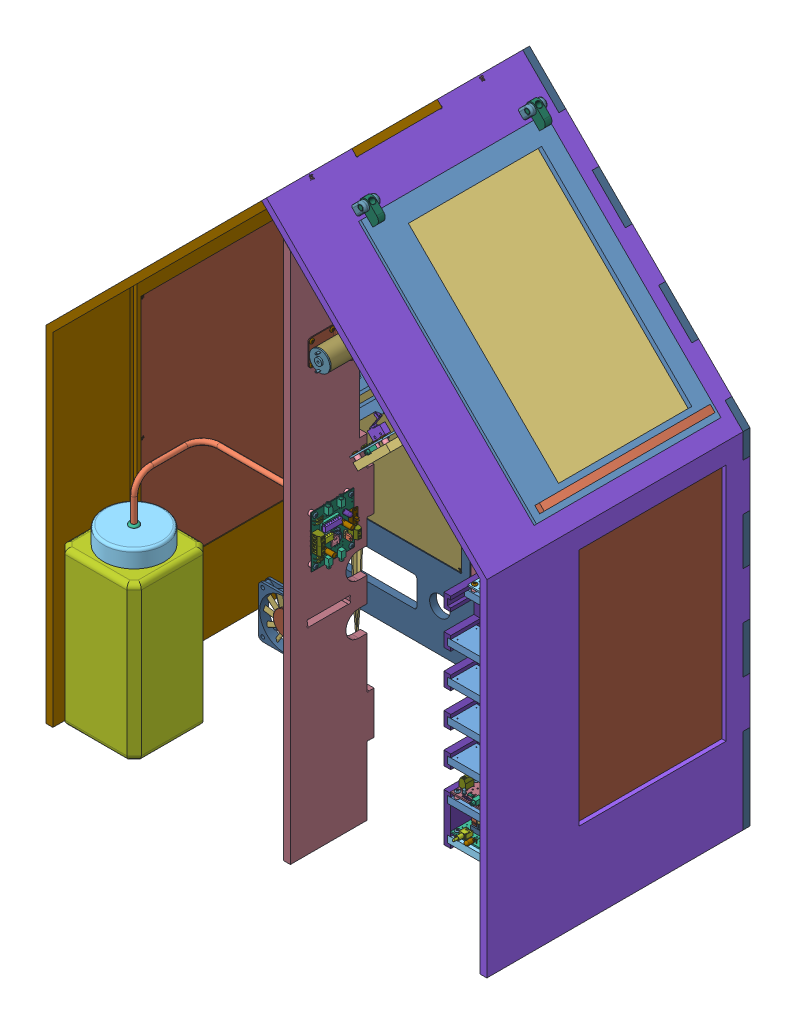
SolidWorks assembly Serre de base VDS, configuration guillotine. Lengths in mm. (continued)
Components (placement in the parent): (continued)
- Cache Oled-2: Cache Oled [Défaut] at (-241.7989 -284.4707 -216) (hidden)
- guillotine-1: guillotine [Défaut] at (-150.376 -16.7665 73.5) (hidden)
- Sonde capteur humidité-1: Sonde capteur humidité [Défaut] at (349.3697 -143.9656 -111.3159) x (1 0 0) z (0 1 0) size (30.38 36.99 53.6) (hidden)
  - Base capteur humidité terre-1: Base capteur humidité terre [Défaut] at (-210.4875 -4.2437 -4) size (29.6 36.6 12.37)
  - Capot capteur humidité terre-1: Capot capteur humidité terre [Défaut] at (-210.4875 -4.2437 32.3863) x (0 0 1) z (-0.999641 -0.026785 0) size (7 29.6 29.6)
  - Tige capteur humidité-1: Tige capteur humidité [Défaut] at (-221.4875 -4.2437 8) x (1 0 0) z (0 1 0) size (3 50 3)
  - Tige capteur humidité-2: Tige capteur humidité [Défaut] at (-199.4875 -4.2437 8) x (1 0 0) z (0 1 0) size (3 50 3)
  - CI capteur humidité terre-1: CI capteur humidité terre [Défaut] at (-210.4875 -4.2437 3) size (25.6 25.6 1.6)
  - Vis 2.2 x 9.5-1: Vis 2.2 x 9.5 [Défaut] at (-210.4875 -4.2437 9.6) x (0.624792 0.780791 0) z (0.780791 -0.624792 0) size (4.27 12.1 4.27)
  - Résistance 75 Kohm Pas de 10-1: Résistance 75 Kohm Pas de 10 [Défaut] at (-210.4875 -12.0088 0.7228) x (1 0 0) z (0 1 0) size (10.5 4.15 2.3)
Mates (geometry in assembly coordinates):
- Coïncidente1: coincident anti-aligned: axis of FONDINTERIEUR-1 through (57.939 191.6778 -4) axis (0 0 1); axis of Rondelle métal 3 x 12-1 through (57.939 191.6778 8.8) axis (0 0 -1)
- Coïncidente2: coincident anti-aligned: axis of Rondelle métal 3 x 12-1 through (57.939 191.6778 8.8) axis (0 0 -1); axis of VIs TC 3 x 13-1 through (57.939 191.6778 -1.7) axis (0 0 1)
- Coïncidente3: coincident anti-aligned: axis of FONDINTERIEUR-1 through (22.5836 156.3225 -4) axis (0 0 1); axis of Rondelle métal 3 x 12-2 through (22.5836 156.3225 8.8) axis (0 0 -1)
- Coïncidente4: coincident anti-aligned: axis of VIs TC 3 x 13-2 through (22.5836 156.3225 -1.7) axis (0 0 1); axis of Rondelle métal 3 x 12-2 through (22.5836 156.3225 8.8) axis (0 0 -1)
- Coïncidente5: coincident aligned: circle of VIs TC 3 x 13-2; plane of Rondelle métal 3 x 12-2 through (22.5836 156.3225 8.8) normal (0 0 1)
- Coïncidente6: coincident anti-aligned: plane of Rondelle métal 3 x 12-1 through (57.939 191.6778 8.8) normal (0 0 1); plane of VIs TC 3 x 13-1 through (57.939 191.6778 8.8) normal (0 0 -1)
- Coïncidente14: coincident anti-aligned: axis of FONDINTERIEUR-1 through (57.939 191.6778 -4) axis (0 0 1); axis of Entretoise CI-1 through (57.939 191.6778 8.1) axis (0 0 -1)
- Coïncidente15: coincident aligned: plane of FONDINTERIEUR-1 through (-297.9367 -225.0262 4) normal (0 0 1); circle of Entretoise CI-1
- Coïncidente16: coincident anti-aligned: axis of FONDINTERIEUR-1 through (22.5836 156.3225 -4) axis (0 0 1); axis of Entretoise CI-2 through (22.5836 156.3225 8.1) axis (0 0 -1)
- Coïncidente17: coincident aligned: plane of FONDINTERIEUR-1 through (-297.9367 -225.0262 4) normal (0 0 1); circle of Entretoise CI-2
- Tangent4: tangent anti-aligned: plane of Crémallière M3-3-1 through (-72.5742 65.3366 12) normal (0.707107 -0.707107 0); cylinder of Entretoise CI-2 through (22.5836 156.3225 8.1) axis (0 0 -1) radius 2.95
- Parallèle1: parallel aligned: plane of FONDINTERIEUR-1 through (-307.876 77.2771 4) normal (-0.707107 0.707107 0); plane of Crémallière M3-3-1 through (-52.7752 102.1062 12) normal (-0.707107 0.707107 0)
- Coïncidente19: coincident anti-aligned: plane of FONDINTERIEUR-1 through (-297.9367 -225.0262 4) normal (0 0 1); plane of Crémallière M3-3-1 through (65.6965 199.3646 4) normal (0 0 -1)
- Coïncidente20: coincident aligned: axis of FONDINTERIEUR-1 through (57.939 191.6778 -4) axis (0 0 1); axis of VIs TC 3 x 13-1 through (57.939 191.6778 -1.7) axis (0 0 1)
- Coïncidente21: coincident anti-aligned: plane of Crémallière M3-3-1 through (-70.4528 63.2153 8) normal (0 0 1); plane of Rondelle métal 3 x 12-1 through (57.939 191.6778 8) normal (0 0 -1)
- Coïncidente22: coincident anti-aligned: plane of Crémallière M3-3-1 through (-70.4528 63.2153 8) normal (0 0 1); plane of Rondelle métal 3 x 12-2 through (22.5836 156.3225 8) normal (0 0 -1)
- Coïncidente23: coincident anti-aligned: plane of FONDINTERIEUR-1 through (62.7794 136.4142 -4) normal (0.707107 -0.707107 0); plane of Prépa 06 module Microrupteur-1/support capteur-1 through (87.5711 161.2058 2.9393) normal (-0.707107 0.707107 0)
- Coïncidente24: coincident anti-aligned: plane of FONDINTERIEUR-1 through (96.8921 167.5269 -4) normal (-0.707107 -0.707107 0); plane of Prépa 06 module Microrupteur-1/support capteur-1 through (95.3921 169.0269 -4) normal (0.707107 0.707107 0)
- Coïncidente25: coincident aligned: plane of FONDINTERIEUR-1 through (-297.9367 -225.0262 -4) normal (0 0 -1); plane of Prépa 06 module Microrupteur-1/support capteur-1 through (95.3921 169.0269 -4) normal (0 0 -1)
- Coïncidente26: coincident anti-aligned: plane of FONDINTERIEUR-1 through (-7.9312 65.7035 -4) normal (0.707107 -0.707107 0); plane of Prépa 06 module Microrupteur-2/support capteur-1 through (16.8604 90.4952 2.9393) normal (-0.707107 0.707107 0)
- Coïncidente27: coincident anti-aligned: plane of FONDINTERIEUR-1 through (26.1815 96.8162 -4) normal (-0.707107 -0.707107 0); plane of Prépa 06 module Microrupteur-2/support capteur-1 through (24.6815 98.3162 -4) normal (0.707107 0.707107 0)
- Coïncidente28: coincident aligned: plane of FONDINTERIEUR-1 through (-297.9367 -225.0262 -4) normal (0 0 -1); plane of Prépa 06 module Microrupteur-2/support capteur-1 through (24.6815 98.3162 -4) normal (0 0 -1)
- Coïncidente29: coincident anti-aligned: axis of FONDINTERIEUR-1 through (-138.876 -138.9656 -4) axis (0 0 1); axis of Ventilateur-1/Cage ventilateur-1 through (-138.876 -138.9656 14.4) axis (0 0 -1)
- Coïncidente30: coincident anti-aligned: axis of FONDINTERIEUR-1 through (-88.876 -138.9656 -4) axis (0 0 1); axis of Ventilateur-1/Cage ventilateur-1 through (-88.876 -138.9656 14.4) axis (0 0 -1)
- Coïncidente31: coincident: plane of FONDINTERIEUR-1 through (-297.9367 -225.0262 4) normal (0 0 1); line of Ventilateur-1/Cage ventilateur-1 through (-143.876 -138.9656 4) axis (0 -1 0)
- Coïncidente32: coincident anti-aligned: axis of Ventilateur-1/Cage ventilateur-1 through (-138.876 -138.9656 14.4) axis (0 0 -1); axis of VIs TC 3 x 13-4 through (-138.876 -138.9656 3.9) axis (0 0 1)
- Coïncidente33: coincident anti-aligned: axis of Ventilateur-1/Cage ventilateur-1 through (-88.876 -138.9656 14.4) axis (0 0 -1); axis of VIs TC 3 x 13-6 through (-88.876 -138.9656 3.9) axis (0 0 1)
- Coïncidente34: coincident anti-aligned: axis of Ventilateur-1/Cage ventilateur-1 through (-88.876 -188.9656 14.4) axis (0 0 -1); axis of VIs TC 3 x 13-7 through (-88.876 -188.9656 3.9) axis (0 0 1)
- Coïncidente35: coincident anti-aligned: axis of Ventilateur-1/Cage ventilateur-1 through (-138.876 -188.9656 14.4) axis (0 0 -1); axis of VIs TC 3 x 13-8 through (-138.876 -188.9656 3.9) axis (0 0 1)
- Coïncidente36: coincident aligned: plane of Ventilateur-1/Cage ventilateur-1 through (-88.876 -138.9656 14.4) normal (0 0 1); circle of VIs TC 3 x 13-8
- Coïncidente37: coincident aligned: plane of Ventilateur-1/Cage ventilateur-1 through (-88.876 -138.9656 14.4) normal (0 0 1); circle of VIs TC 3 x 13-4
- Coïncidente38: coincident aligned: plane of Ventilateur-1/Cage ventilateur-1 through (-88.876 -138.9656 14.4) normal (0 0 1); circle of VIs TC 3 x 13-6
- Coïncidente39: coincident aligned: plane of Ventilateur-1/Cage ventilateur-1 through (-88.876 -138.9656 14.4) normal (0 0 1); circle of VIs TC 3 x 13-7
- Coïncidente40: coincident aligned: axis of FONDINTERIEUR-1 through (8.418 76.3959 4) axis (0 0 -1); axis of VIS TORCX TF 3 X 19-2 through (8.418 76.3959 12.4885) axis (0 0 -1)
- Coïncidente41: coincident aligned: plane of FONDINTERIEUR-1 through (-297.9367 -225.0262 -4) normal (0 0 -1); plane of VIS TORCX TF 3 X 19-2 through (7.3455 78.9824 -4) normal (0 0 -1)
- Coïncidente42: coincident aligned: axis of FONDINTERIEUR-1 through (79.1287 147.1066 4) axis (0 0 -1); axis of VIS TORCX TF 3 X 19-1 through (79.1287 147.1066 12.4885) axis (0 0 -1)
- Coïncidente43: coincident aligned: plane of FONDINTERIEUR-1 through (-297.9367 -225.0262 -4) normal (0 0 -1); plane of VIS TORCX TF 3 X 19-1 through (78.0561 149.693 -4) normal (0 0 -1)
- Coïncidente44: coincident anti-aligned: plane of FONDINTERIEUR-1 through (-26.876 223.1558 -4) normal (-1 0 0); plane of Prépa 02 renfort arrière-1/renfortarriere-1 through (-26.876 272.0951 2.9393) normal (1 0 0)
- Coïncidente45: coincident anti-aligned: plane of FONDINTERIEUR-1 through (-28.9973 271.0344 -4) normal (0 -1 0); plane of Prépa 02 renfort arrière-1/renfortarriere-1 through (-26.876 271.0344 -4) normal (0 1 0)
- Coïncidente46: coincident aligned: plane of FONDINTERIEUR-1 through (-297.9367 -225.0262 -4) normal (0 0 -1); plane of Prépa 02 renfort arrière-1/renfortarriere-1 through (-26.876 221.1086 -4) normal (0 0 -1)
- Coïncidente47: coincident anti-aligned: plane of FONDINTERIEUR-1 through (-56.9973 -85.9656 -4) normal (0 -1 0); plane of étagèrebrumi-1 through (-297.9367 -85.9656 72.872) normal (0 1 0)
- Coïncidente48: coincident anti-aligned: plane of FONDINTERIEUR-1 through (-54.876 -88.0869 -4) normal (-1 0 0); plane of étagèrebrumi-1 through (-54.876 -85.9656 1.8787) normal (1 0 0)
- Coïncidente49: coincident aligned: plane of FONDINTERIEUR-1 through (-297.9367 -225.0262 -4) normal (0 0 -1); plane of étagèrebrumi-1 through (-54.876 -85.9656 -4) normal (0 0 -1)
- Coïncidente50: coincident anti-aligned: axis of FONDINTERIEUR-1 through (-30.876 -315.9656 -4) axis (0 0 1); axis of VIS TORCX TF 3 X 19-3 through (-30.876 -315.9656 12.4885) axis (0 0 -1)
- Coïncidente51: coincident aligned: plane of FONDINTERIEUR-1 through (-297.9367 -225.0262 -4) normal (0 0 -1); plane of VIS TORCX TF 3 X 19-3 through (-31.2492 -313.1905 -4) normal (0 0 -1)
- Coïncidente52: coincident anti-aligned: axis of FONDINTERIEUR-1 through (-30.876 -274.5499 -4) axis (0 0 1); axis of VIS TORCX TF 3 X 19-4 through (-30.876 -274.5499 12.4885) axis (0 0 -1)
- Coïncidente53: coincident aligned: plane of FONDINTERIEUR-1 through (-297.9367 -225.0262 -4) normal (0 0 -1); plane of VIS TORCX TF 3 X 19-4 through (-31.2492 -271.7749 -4) normal (0 0 -1)
- Coïncidente54: coincident anti-aligned: axis of FONDINTERIEUR-1 through (-169.876 -89.9656 -4) axis (0 0 1); axis of VIS TORCX TF 3 X 19-5 through (-169.876 -89.9656 12.4885) axis (0 0 -1)
- Coïncidente55: coincident aligned: plane of FONDINTERIEUR-1 through (-297.9367 -225.0262 -4) normal (0 0 -1); plane of VIS TORCX TF 3 X 19-5 through (-170.2492 -87.1905 -4) normal (0 0 -1)
- Coïncidente56: coincident anti-aligned: axis of FONDINTERIEUR-1 through (-30.876 -27.0369 -4) axis (0 0 1); axis of VIS TORCX TF 3 X 19-6 through (-30.876 -27.0369 12.4885) axis (0 0 -1)
- Coïncidente57: coincident aligned: plane of FONDINTERIEUR-1 through (-297.9367 -225.0262 -4) normal (0 0 -1); plane of VIS TORCX TF 3 X 19-6 through (-31.2492 -24.2619 -4) normal (0 0 -1)
- Coïncidente58: coincident anti-aligned: axis of FONDINTERIEUR-1 through (-30.876 278.5344 -4) axis (0 0 1); axis of VIS TORCX TF 3 X 19-7 through (-30.876 278.5344 12.4885) axis (0 0 -1)
- Coïncidente59: coincident aligned: plane of FONDINTERIEUR-1 through (-297.9367 -225.0262 -4) normal (0 0 -1); plane of VIS TORCX TF 3 X 19-7 through (-31.2492 281.3095 -4) normal (0 0 -1)
- Coïncidente60: coincident anti-aligned: plane of FONDINTERIEUR-1 through (-296.876 -226.0869 4) normal (-1 0 0); plane of Coté gauche serre-1 through (-296.876 -275.0426 -2.9402) normal (1 0 0)
- Coïncidente61: coincident anti-aligned: plane of FONDINTERIEUR-1 through (-298.9973 -273.9656 4) normal (0 1 0); plane of Coté gauche serre-1 through (-296.876 -273.9656 1.8944) normal (0 -1 0)
- Coïncidente62: coincident anti-aligned: plane of FONDINTERIEUR-1 through (-297.9367 -225.0262 -4) normal (0 0 -1); plane of Coté gauche serre-1 through (-296.876 -323.9656 -4) normal (0 0 1)
- Coïncidente63: coincident anti-aligned: plane of FONDINTERIEUR-1 through (-154.876 -315.9656 -4) normal (0 -1 0); plane of suportbloceau-1 through (-297.9367 -315.9656 75.0607) normal (0 1 0)
- Coïncidente64: coincident anti-aligned: plane of FONDINTERIEUR-1 through (-204.876 -318.0869 -4) normal (1 0 0); plane of suportbloceau-1 through (-204.876 -315.9656 -4) normal (-1 0 0)
- Coïncidente65: coincident aligned: plane of FONDINTERIEUR-1 through (-297.9367 -225.0262 -4) normal (0 0 -1); plane of suportbloceau-1 through (-154.876 -315.9656 -4) normal (0 0 -1)
- Coïncidente66: coincident anti-aligned: plane of FONDINTERIEUR-1 through (-95.876 -28.0869 4) normal (1 0 0); plane of Coté support brumisateur-1 through (-95.876 -24.9049 2.9393) normal (-1 0 0)
- Coïncidente67: coincident anti-aligned: plane of FONDINTERIEUR-1 through (-89.9973 -65.9656 4) normal (0 1 0); plane of Coté support brumisateur-1 through (-95.876 -65.9656 -4) normal (0 -1 0)
- Coïncidente68: coincident aligned: plane of FONDINTERIEUR-1 through (-297.9367 -225.0262 -4) normal (0 0 -1); plane of Coté support brumisateur-1 through (-95.876 -25.9656 -4) normal (0 0 -1)
- Coïncidente69: coincident anti-aligned: plane of FONDINTERIEUR-1 through (-212.876 -28.0869 4) normal (1 0 0); plane of Coté support brumisateur-2 through (-212.876 -24.9049 2.9393) normal (-1 0 0)
- Coïncidente70: coincident anti-aligned: plane of FONDINTERIEUR-1 through (-210.7547 -65.9656 4) normal (0 1 0); plane of Coté support brumisateur-2 through (-212.876 -65.9656 -4) normal (0 -1 0)
- Coïncidente71: coincident aligned: plane of FONDINTERIEUR-1 through (-297.9367 -225.0262 -4) normal (0 0 -1); plane of Coté support brumisateur-2 through (-212.876 -25.9656 -4) normal (0 0 -1)
- Coïncidente72: coincident anti-aligned: plane of FONDINTERIEUR-1 through (-189.2547 -195.9656 -4) normal (0 1 0); plane of Renfort bidon-1 through (-192.4367 -195.9656 2.9393) normal (0 -1 0)
- Coïncidente73: coincident anti-aligned: plane of FONDINTERIEUR-1 through (-191.376 -190.0869 -4) normal (1 0 0); plane of Renfort bidon-1 through (-191.376 -187.9656 1.8787) normal (-1 0 0)
- Coïncidente74: coincident aligned: plane of FONDINTERIEUR-1 through (-297.9367 -225.0262 -4) normal (0 0 -1); plane of Renfort bidon-1 through (-191.376 -187.9656 -4) normal (0 0 -1)
- Coïncidente75: coincident aligned: axis of FONDINTERIEUR-1 through (-198.876 -191.9656 4) axis (0 0 -1); axis of VIS TORCX TF 3 X 19-12 through (-198.876 -191.9656 12.4885) axis (0 0 -1)
- Coïncidente76: coincident aligned: plane of FONDINTERIEUR-1 through (-297.9367 -225.0262 -4) normal (0 0 -1); plane of VIS TORCX TF 3 X 19-12 through (-199.9485 -189.3791 -4) normal (0 0 -1)
- Coïncidente77: coincident aligned: axis of FONDINTERIEUR-1 through (-164.4919 -191.9656 4) axis (0 0 -1); axis of VIS TORCX TF 3 X 19-13 through (-164.4919 -191.9656 12.4885) axis (0 0 -1)
- Coïncidente78: coincident aligned: plane of FONDINTERIEUR-1 through (-297.9367 -225.0262 -4) normal (0 0 -1); plane of VIS TORCX TF 3 X 19-13 through (-165.5644 -189.3791 -4) normal (0 0 -1)
- Coïncidente79: coincident aligned: axis of FONDINTERIEUR-1 through (-208.876 -75.9656 4) axis (0 0 -1); axis of VIS TORCX TF 3 X 19-14 through (-208.876 -75.9656 12.4885) axis (0 0 -1)
- Coïncidente80: coincident aligned: plane of FONDINTERIEUR-1 through (-297.9367 -225.0262 -4) normal (0 0 -1); plane of VIS TORCX TF 3 X 19-14 through (-209.9485 -73.3791 -4) normal (0 0 -1)
- Coïncidente81: coincident aligned: axis of FONDINTERIEUR-1 through (-208.876 -16.4656 4) axis (0 0 -1); axis of VIS TORCX TF 3 X 19-15 through (-208.876 -16.4656 12.4885) axis (0 0 -1)
- Coïncidente82: coincident aligned: plane of FONDINTERIEUR-1 through (-297.9367 -225.0262 -4) normal (0 0 -1); plane of VIS TORCX TF 3 X 19-15 through (-209.9485 -13.8791 -4) normal (0 0 -1)
- Coïncidente83: coincident aligned: axis of FONDINTERIEUR-1 through (-91.876 -75.9656 4) axis (0 0 -1); axis of VIS TORCX TF 3 X 19-16 through (-91.876 -75.9656 12.4885) axis (0 0 -1)
- Coïncidente84: coincident aligned: plane of FONDINTERIEUR-1 through (-297.9367 -225.0262 -4) normal (0 0 -1); plane of VIS TORCX TF 3 X 19-16 through (-92.9485 -73.3791 -4) normal (0 0 -1)
- Coïncidente85: coincident aligned: axis of FONDINTERIEUR-1 through (-91.876 -15.9656 4) axis (0 0 -1); axis of VIS TORCX TF 3 X 19-17 through (-91.876 -15.9656 12.4885) axis (0 0 -1)
- Coïncidente86: coincident aligned: plane of FONDINTERIEUR-1 through (-297.9367 -225.0262 -4) normal (0 0 -1); plane of VIS TORCX TF 3 X 19-17 through (-92.9485 -13.3791 -4) normal (0 0 -1)
- Coïncidente87: coincident aligned: axis of Coté gauche serre-1 through (-296.876 -89.9656 48.9996) axis (-1 0 0); axis of VIS TORCX TF 3 X 19-18 through (-288.3875 -89.9656 48.9996) axis (-1 0 0)
- Coïncidente88: coincident aligned: plane of Coté gauche serre-1 through (-304.876 -275.0426 -2.9402) normal (-1 0 0); plane of VIS TORCX TF 3 X 19-18 through (-304.876 -87.1656 48.9996) normal (-1 0 0)
- Coïncidente89: coincident aligned: axis of Coté gauche serre-1 through (-296.876 -248.9656 -0.0009) axis (-1 0 0); axis of VIS TORCX TF 3 X 19-25 through (-288.3875 -248.9656 -0.0009) axis (-1 0 0)
- Coïncidente90: coincident aligned: plane of Coté gauche serre-1 through (-304.876 -275.0426 -2.9402) normal (-1 0 0); plane of VIS TORCX TF 3 X 19-25 through (-304.876 -246.1656 -0.0009) normal (-1 0 0)
- Coïncidente91: coincident aligned: axis of suportbloceau-1 through (-300.876 -315.9656 49) axis (0 -1 0); axis of VIS TORCX TF 3 X 19-26 through (-300.876 -307.477 49) axis (0 -1 0)
- Coïncidente92: coincident aligned: plane of suportbloceau-1 through (-297.9367 -323.9656 75.0607) normal (0 -1 0); plane of VIS TORCX TF 3 X 19-26 through (-299.1327 -323.9656 51.1911) normal (0 -1 0)
- Coïncidente93: coincident aligned: axis of suportbloceau-1 through (-271.876 -315.9656 0) axis (0 -1 0); axis of VIS TORCX TF 3 X 19-29 through (-271.876 -307.477 0) axis (0 -1 0)
- Coïncidente94: coincident aligned: plane of suportbloceau-1 through (-297.9367 -323.9656 75.0607) normal (0 -1 0); plane of VIS TORCX TF 3 X 19-29 through (-270.1327 -323.9656 2.1911) normal (0 -1 0)
- Coïncidente95: coincident aligned: axis of suportbloceau-1 through (-179.876 -315.9656 0) axis (0 -1 0); axis of VIS TORCX TF 3 X 19-30 through (-179.876 -307.477 0) axis (0 -1 0)
- Coïncidente96: coincident aligned: plane of suportbloceau-1 through (-297.9367 -323.9656 75.0607) normal (0 -1 0); plane of VIS TORCX TF 3 X 19-30 through (-178.1327 -323.9656 2.1911) normal (0 -1 0)
- Coïncidente103: coincident anti-aligned: plane of FONDINTERIEUR-1 through (187.124 -226.0869 4) normal (1 0 0); plane of Coté droit serre-1 through (187.124 -275.0262 -2.9393) normal (-1 0 0)
- Coïncidente104: coincident anti-aligned: plane of FONDINTERIEUR-1 through (195.124 -223.9656 4) normal (0 -1 0); plane of Coté droit serre-1 through (195.124 -223.9656 46) normal (0 1 0)
- Coïncidente105: coincident anti-aligned: plane of FONDINTERIEUR-1 through (-297.9367 -225.0262 -4) normal (0 0 -1); plane of Coté droit serre-1 through (195.124 -323.9656 -4) normal (0 0 1)
- Coïncidente114: coincident anti-aligned: axis of Coté droit serre-1 through (195.124 -248.9656 0) axis (-1 0 0); axis of VIS TORCX TF 3 X 19-35 through (178.6355 -248.9656 0) axis (1 0 0)
- Coïncidente115: coincident aligned: plane of Coté droit serre-1 through (195.124 -275.0262 -2.9393) normal (1 0 0); plane of VIS TORCX TF 3 X 19-35 through (195.124 -246.2177 -0.5377) normal (1 0 0)
- Coïncidente116: coincident anti-aligned: plane of FONDINTERIEUR-1 through (48.6689 -231.9656 -4) normal (0 1 0); plane of Poutre fond-1 through (-276.7874 -231.9656 -2.9393) normal (0 -1 0)
- Coïncidente117: coincident anti-aligned: plane of FONDINTERIEUR-1 through (0.7902 -229.8442 -4) normal (1 0 0); plane of Poutre fond-1 through (0.7902 -223.9656 4) normal (-1 0 0)
- Coïncidente118: coincident anti-aligned: plane of FONDINTERIEUR-1 through (-297.9367 -225.0262 -4) normal (0 0 -1); plane of Poutre fond-1 through (-108.4209 -223.9656 -4) normal (0 0 1)
- Coïncidente119: coincident aligned: axis of FONDINTERIEUR-1 through (103.3825 -227.9656 -4) axis (0 0 1); axis of VIS TORCX TF 3 X 19-49 through (103.3825 -227.9656 -12.4885) axis (0 0 1)
- Coïncidente120: coincident aligned: plane of FONDINTERIEUR-1 through (-297.9367 -225.0262 4) normal (0 0 1); plane of VIS TORCX TF 3 X 19-49 through (103.3825 -225.1656 4) normal (0 0 1)
- Coïncidente121: coincident aligned: axis of FONDINTERIEUR-1 through (-54.876 -227.9656 -4) axis (0 0 1); axis of VIS TORCX TF 3 X 19-37 through (-54.876 -227.9656 -12.4885) axis (0 0 1)
- Coïncidente122: coincident aligned: plane of FONDINTERIEUR-1 through (-297.9367 -225.0262 4) normal (0 0 1); plane of VIS TORCX TF 3 X 19-37 through (-54.876 -225.1656 4) normal (0 0 1)
- Coïncidente124: coincident aligned: axis of FONDINTERIEUR-1 through (-213.1345 -227.9656 -4) axis (0 0 1); axis of VIS TORCX TF 3 X 19-36 through (-213.1345 -227.9656 -12.4885) axis (0 0 1)
- Coïncidente125: coincident aligned: plane of FONDINTERIEUR-1 through (-297.9367 -225.0262 4) normal (0 0 1); plane of VIS TORCX TF 3 X 19-36 through (-213.1345 -225.1656 4) normal (0 0 1)
- Coïncidente126: coincident anti-aligned: plane of Poutre fond-1 through (-296.876 -223.9656 -13) normal (0 0 -1); plane of Poutre plateau-1 through (79.7388 -229.6404 -13) normal (0 0 1)
- Coïncidente127: coincident aligned: plane of Coté droit serre-1 through (195.124 -275.0262 -2.9393) normal (1 0 0); plane of Poutre plateau-1 through (195.124 -223.9656 -21) normal (1 0 0)
- Coïncidente128: coincident anti-aligned: plane of Coté droit serre-1 through (195.124 -243.9656 -18.9697) normal (0 1 0); plane of Poutre plateau-1 through (195.124 -243.9656 -21) normal (0 -1 0)
- Coïncidente129: coincident anti-aligned: plane of Coté droit serre-1 through (195.124 -291.8442 -198) normal (0 0 -1); plane of façadeporteplateau-1 through (188.1847 -295.0262 -198) normal (0 0 1)
- Coïncidente130: coincident aligned: plane of Coté droit serre-1 through (195.124 -275.0262 -2.9393) normal (1 0 0); plane of façadeporteplateau-1 through (195.124 -253.9656 -198) normal (1 0 0)
- Coïncidente131: coincident aligned: plane of Coté droit serre-1 through (195.124 -223.9656 -21.091) normal (0 1 0); plane of façadeporteplateau-1 through (-296.876 -223.9656 -198) normal (0 1 0)
- Coïncidente132: coincident anti-aligned: axis of Coté droit serre-1 through (195.124 -238.9656 -202) axis (-1 0 0); axis of VIS TORCX TF 3 X 19-40 through (178.6355 -238.9656 -202) axis (1 0 0)
- Coïncidente133: coincident aligned: plane of Coté droit serre-1 through (195.124 -275.0262 -2.9393) normal (1 0 0); plane of VIS TORCX TF 3 X 19-40 through (195.124 -236.1656 -202) normal (1 0 0)
- Coïncidente134: coincident anti-aligned: axis of Coté droit serre-1 through (195.124 -308.9656 -202) axis (-1 0 0); axis of VIS TORCX TF 3 X 19-39 through (178.6355 -308.9656 -202) axis (1 0 0)
- Coïncidente135: coincident aligned: plane of Coté droit serre-1 through (195.124 -275.0262 -2.9393) normal (1 0 0); plane of VIS TORCX TF 3 X 19-39 through (195.124 -306.1656 -202) normal (1 0 0)
- Coïncidente136: coincident aligned: axis of façadeporteplateau-1 through (191.124 -273.9656 -198) axis (0 0 -1); axis of VIS TORCX TF 3 X 19-38 through (191.124 -273.9656 -189.5115) axis (0 0 -1)
- Coïncidente137: coincident aligned: plane of façadeporteplateau-1 through (188.1847 -295.0262 -206) normal (0 0 -1); plane of VIS TORCX TF 3 X 19-38 through (190.0515 -271.3791 -206) normal (0 0 -1)
- Coïncidente138: coincident aligned: axis of façadeporteplateau-1 through (-300.876 -273.9656 -198) axis (0 0 -1); axis of VIS TORCX TF 3 X 19-43 through (-300.876 -273.9656 -189.5115) axis (0 0 -1)
- Coïncidente139: coincident aligned: plane of façadeporteplateau-1 through (188.1847 -295.0262 -206) normal (0 0 -1); plane of VIS TORCX TF 3 X 19-43 through (-301.9485 -271.3791 -206) normal (0 0 -1)
- Coïncidente140: coincident aligned: axis of Coté gauche serre-1 through (-296.876 -238.9737 -202) axis (-1 0 0); axis of VIS TORCX TF 3 X 19-44 through (-288.3875 -238.9737 -202) axis (-1 0 0)
- Coïncidente141: coincident aligned: plane of Coté gauche serre-1 through (-304.876 -275.0426 -2.9402) normal (-1 0 0); plane of VIS TORCX TF 3 X 19-44 through (-304.876 -236.1737 -202) normal (-1 0 0)
- Coïncidente142: coincident aligned: axis of Coté gauche serre-1 through (-296.876 -308.9656 -202) axis (-1 0 0); axis of VIS TORCX TF 3 X 19-45 through (-288.3875 -308.9656 -202) axis (-1 0 0)
- Coïncidente143: coincident aligned: plane of Coté gauche serre-1 through (-304.876 -275.0426 -2.9402) normal (-1 0 0); plane of VIS TORCX TF 3 X 19-45 through (-304.876 -306.1656 -202) normal (-1 0 0)
- Coïncidente144: coincident anti-aligned: plane of FONDINTERIEUR-1 through (112.8547 -40.3939 -4) normal (1 0 0); plane of Sous ensemble Rack module-1/rack coté gauche-1 through (112.8547 -36.9223 2.9393) normal (-1 0 0)
- Coïncidente145: coincident anti-aligned: plane of FONDINTERIEUR-1 through (176.9761 -37.9656 -4) normal (0 -1 0); plane of Sous ensemble Rack module-1/rack coté droit-1 through (182.8547 -37.9656 1.8787) normal (0 1 0)
- Coïncidente146: coincident aligned: plane of FONDINTERIEUR-1 through (-297.9367 -225.0262 -4) normal (0 0 -1); plane of Sous ensemble Rack module-1/rack coté droit-1 through (182.8547 -37.9656 -4) normal (0 0 -1)
- Coïncidente147: coincident aligned: axis of FONDINTERIEUR-1 through (178.8547 -145.9656 4) axis (0 0 -1); axis of VIS TORCX TF 3 X 19-50 through (178.8547 -145.9656 12.4885) axis (0 0 -1)
- Coïncidente148: coincident aligned: plane of FONDINTERIEUR-1 through (-297.9367 -225.0262 -4) normal (0 0 -1); plane of VIS TORCX TF 3 X 19-50 through (177.7822 -143.3791 -4) normal (0 0 -1)
- Coïncidente149: coincident aligned: axis of FONDINTERIEUR-1 through (116.8547 -145.9656 4) axis (0 0 -1); axis of VIS TORCX TF 3 X 19-51 through (116.8547 -145.9656 12.4885) axis (0 0 -1)
- Coïncidente150: coincident aligned: plane of FONDINTERIEUR-1 through (-297.9367 -225.0262 -4) normal (0 0 -1); plane of VIS TORCX TF 3 X 19-51 through (115.7822 -143.3791 -4) normal (0 0 -1)
- Coïncidente151: coincident anti-aligned: axis of FONDINTERIEUR-1 through (178.8547 -7.9656 -4) axis (0 0 1); axis of VIS TORCX TF 3 X 19-52 through (178.8547 -7.9656 12.4885) axis (0 0 -1)
- Coïncidente152: coincident aligned: plane of FONDINTERIEUR-1 through (-297.9367 -225.0262 -4) normal (0 0 -1); plane of VIS TORCX TF 3 X 19-52 through (177.7822 -5.3791 -4) normal (0 0 -1)
- Coïncidente153: coincident anti-aligned: axis of FONDINTERIEUR-1 through (116.8547 -7.9656 -4) axis (0 0 1); axis of VIS TORCX TF 3 X 19-53 through (116.8547 -7.9656 12.4885) axis (0 0 -1)
- Coïncidente154: coincident aligned: plane of FONDINTERIEUR-1 through (-297.9367 -225.0262 -4) normal (0 0 -1); plane of VIS TORCX TF 3 X 19-53 through (115.7822 -5.3791 -4) normal (0 0 -1)
- Coïncidente163: coincident aligned: axis of FONDINTERIEUR-1 through (-255.126 -66.1655 -4) axis (0 0 1); axis of Sous ensemble Arrosage-1/Tuyau gouteur-1 through (-255.126 -66.1655 -11.25) axis (0 0 1)
- Coïncidente164: coincident anti-aligned: plane of suportbloceau-1 through (-297.9367 -315.9656 75.0607) normal (0 1 0); plane of Sous ensemble Arrosage-1/Reservoir 1,25L-1 through (-272.5 -315.9655 45.1435) normal (0 -1 0)
- Coïncidente168: coincident anti-aligned: plane of FONDINTERIEUR-1 through (-297.9367 -225.0262 4) normal (0 0 1); plane of Sous ensemble Arrosage-1/Reservoir 1,25L-1 through (-299.876 -315.9655 4) normal (0 0 -1)
- Coïncidente169: coincident anti-aligned: plane of Coté droit serre-1 through (191.124 -234.9049 -200.9393) normal (-1 0 0); plane of plateau base-1 through (191.124 -227.9656 -202) normal (1 0 0)
- Coïncidente170: coincident anti-aligned: plane of Coté droit serre-1 through (191.124 -235.9656 -199.8787) normal (0 1 0); plane of plateau base-1 through (-230.7684 -235.9656 -41.3241) normal (0 -1 0)
- Coïncidente173: coincident anti-aligned: plane of Poutre plateau-1 through (79.7388 -229.6404 -17) normal (0 0 -1); plane of plateau base-1 through (-300.876 -227.9656 -17) normal (0 0 1)
- Coïncidente178: coincident anti-aligned: axis of FONDINTERIEUR-1 through (152.3558 6.7126 -4) axis (0 0 1); axis of fondcuivré-1 through (152.3558 6.7126 -4) axis (0 0 -1)
- Coïncidente179: coincident anti-aligned: plane of FONDINTERIEUR-1 through (-297.9367 -225.0262 -4) normal (0 0 -1); plane of fondcuivré-1 through (-208.3657 -251.1382 -4) normal (0 0 1)
- Parallèle5: parallel anti-aligned: line of FONDINTERIEUR-1 through (-62.876 322.2771 -4) axis (1 0 0); line of fondcuivré-1 through (-29.876 291.0344 -5) axis (-1 0 0)
- Coïncidente180: coincident anti-aligned: plane of façadeporteplateau-1 through (188.1847 -295.0262 -206) normal (0 0 -1); plane of Capot complet-1/Capotfaçade-1 through (-305.9367 -222.9049 -206) normal (0 0 1)
- Coïncidente181: coincident aligned: plane of façadeporteplateau-1 through (-296.876 -323.9656 -198) normal (0 -1 0); plane of Capot complet-1/Capotfaçade-1 through (-312.876 -323.9656 -206) normal (0 -1 0)
- Coïncidente182: coincident anti-aligned: line of Coté droit serre-1 through (195.124 -323.9656 -4) axis (0 0 -1); line of Capot complet-1/Capot coté droit-1 through (195.124 -323.9656 -206) axis (0 0 1)
- Coïncidente185: coincident anti-aligned: plane of Capot complet-1/Capotfaçade-1 through (-305.9367 -222.9049 -214) normal (0 0 -1); plane of Cache Oled-2 through (-241.7989 -284.4707 -214) normal (0 0 1)
- Coïncidente186: coincident aligned: line of guillotine-1 through (-87.876 -25.9656 81.5) axis (0 0 -1); line of Coté support brumisateur-1 through (-87.876 -25.9656 82) axis (0 0 -1)
- Coïncidente187: coincident aligned: plane of Coté support brumisateur-1 through (-87.876 -24.9049 2.9393) normal (1 0 0); plane of guillotine-1 through (-87.876 -7.5675 81.5) normal (1 0 0)
- Coïncidente189: coincident anti-aligned: plane of Coté support brumisateur-1 through (-95.876 -25.9656 73.5) normal (0 0 1); plane of guillotine-1 through (-150.376 149.9325 73.5) normal (0 0 -1)
- Distance1: distance = 80 mm anti-aligned: plane of Sonde capteur humidité-1/Base capteur humidité terre-1 through (138.8822 -147.9656 -107.0722) normal (0 -1 0); plane of plateau base-1 through (-230.7684 -227.9656 -41.3241) normal (0 1 0)
